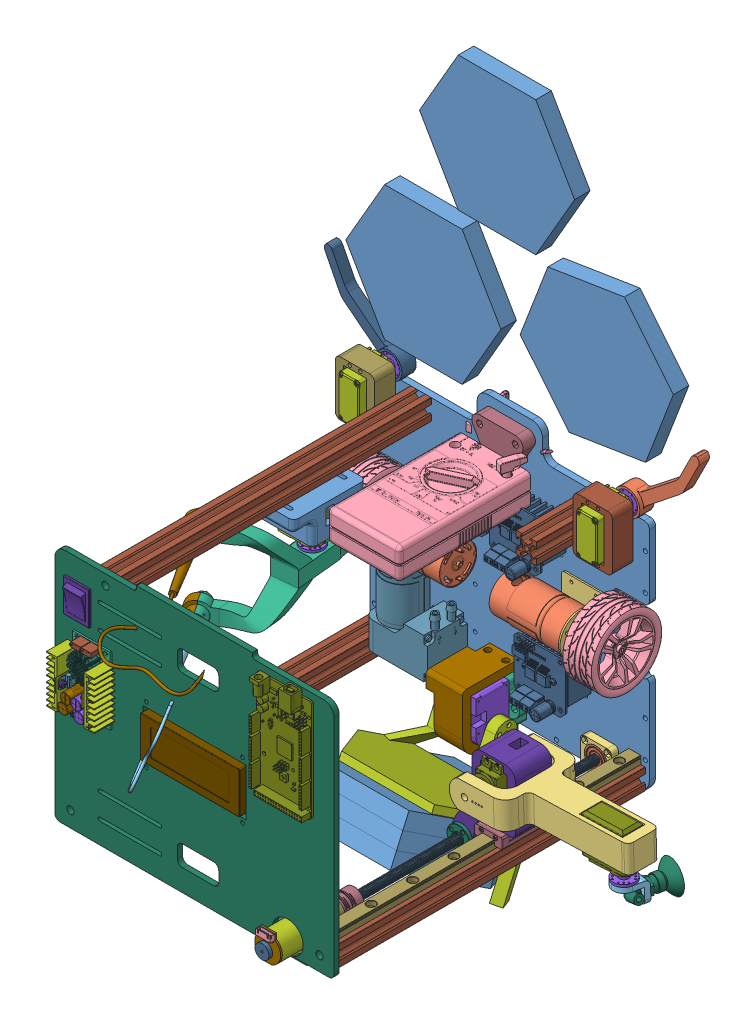
SolidWorks assembly conception_grand_robot_version_final, configuration Default. Lengths in mm.
Overall size (518.63 617.26 405.48).
409 component instances, 143 part files, 130 mates.
Components (placement in the parent):
- base-1: base [Default] at (122.9528 157.5833 221.7888) size (270 260 6)
- assemblage_motor_complet-1: assemblage_motor_complet [Default] at (122.8124 108.9997 302.4952) x (0 1 0) z (-1 0 0) size (92.56 92.56 113.78)
  - Motor 300RPM-1: Motor 300RPM [Default] at (60.9586 47.2064 18.9845) size (37 37 94.88)
  - BAse motor-1: BAse motor [Predeterminado] at (28.5836 74.7064 94.3595) x (1 0 0) z (0 0 -1) size (40 46 43)
  - wheel-1: wheel [Default] at (48.5836 55.7064 86.8847) x (-0.872522 -0.488575 0) z (-0.488575 0.872522 0) size (68 29.75 68)
  - accoupelement court-1: accoupelement court [Default] at (48.5836 55.7064 101.8595) x (-0.320714 0.947176 0) z (0 0 1) size (13.86 12 18)
- assemblage_motor_complet-2: assemblage_motor_complet [Default] at (123.0933 206.1669 302.4952) x (0 -1 0) z (1 0 0) size (92.56 92.56 113.78)
  - Motor 300RPM-1: Motor 300RPM [Default] at (60.9586 47.2064 18.9845) size (37 37 94.88)
  - BAse motor-1: BAse motor [Predeterminado] at (28.5836 74.7064 94.3595) x (1 0 0) z (0 0 -1) size (40 46 43)
  - wheel-1: wheel [Default] at (48.5836 55.7064 86.8847) x (-0.872522 -0.488575 0) z (-0.488575 0.872522 0) size (68 29.75 68)
  - accoupelement court-1: accoupelement court [Default] at (48.5836 55.7064 101.8595) x (-0.320714 0.947176 0) z (0 0 1) size (13.86 12 18)
- bille porteuse-1: bille porteuse [Défaut] at (122.9528 39.4366 218.2888) x (-1 0 0) z (0 1 0) size (52.5 22.5 43)
  - Robot2015_support bille porteuse_arriere-1: Robot2015_support bille porteuse_arriere [Défaut] at (0 9.5 0) size (52.5 22.5 43)
- pince 3-1: pince 3 [Default] at (122.9528 -18.4476 239.2747) x (1 0 0) z (0 0.403318 0.91506) size (152.18 120 85.13)
- Servo-1: Servo [Default] at (139.2028 54.0833 260.7888) x (0 0 -1) z (-1 0 0) size (32 43 41.5)
- TABLE_2021.step-1: TABLE_2021.step [Default] at (1982.9528 825.0833 212.7888) x (0 -1 0) z (0 0 1) size (3306.25 2336 1029.4) (hidden)
  - BaseTable.step-1: BaseTable.step [Défaut] at (0 0 -22) x (1 0 0) z (0 -1 0) size (3288 1022 2266)
    - Edge Beacon Right.step-1: Edge Beacon Right.step [Défaut] at (-884.0915 354.4211 0) x (1 0 0) z (0 1 0) size (122 122 92)
      - EdgeBeacons_Base.step-1: EdgeBeacons_Base.step [Défaut] at (3967.0915 -989 -332.4211) x (0 -1 0) z (1 0 0) size (122 22 122)
      - EdgeBeacons_SmallBorder.step-1: EdgeBeacons_SmallBorder.step [Défaut] at (4028.0915 -950 -332.4211) x (0 1 0) z (1 0 0) size (22 70 100)
      - EdgeBeacons_LargeBorder.step-1: EdgeBeacons_LargeBorder.step [Défaut] at (3906.0915 -1050 -332.4211) x (1 0 0) z (0 -1 0) size (22 70 122)
    - Edge Beacon Left.step-1: Edge Beacon Left.step [Défaut] at (-1609.4995 44.4467 0) x (1 0 0) z (0 1 0) size (122 122 92)
      - EdgeBeacons_Base.step-1: EdgeBeacons_Base.step [Défaut] at (1526.4995 -39 -44.4467) x (0 -1 0) z (-1 0 0) size (122 22 122)
      - EdgeBeacons_LargeBorder.step-1: EdgeBeacons_LargeBorder.step [Défaut] at (1565.4995 -100 -22.4467) x (1 0 0) z (0 -1 0) size (22 70 122)
      - EdgeBeacons_SmallBorder.step-1: EdgeBeacons_SmallBorder.step [Défaut] at (1465.4995 22 -22.4467) x (0 -1 0) z (-1 0 0) size (22 70 100)
    - Edge Beacon Right_1.step-1: Edge Beacon Right_1.step [Défaut] at (-884.0915 354.4211 0) x (1 0 0) z (0 1 0) size (122 122 92)
      - EdgeBeacons_Base.step-1: EdgeBeacons_Base.step [Défaut] at (3967.0915 -39 -332.4211) x (0 -1 0) z (1 0 0) size (122 22 122)
      - EdgeBeacons_SmallBorder.step-1: EdgeBeacons_SmallBorder.step [Défaut] at (4028.0915 0 -332.4211) x (0 1 0) z (1 0 0) size (22 70 100)
      - EdgeBeacons_LargeBorder.step-1: EdgeBeacons_LargeBorder.step [Défaut] at (3906.0915 -100 -332.4211) x (1 0 0) z (0 -1 0) size (22 70 122)
    - Edge Beacon Right_2.step-1: Edge Beacon Right_2.step [Défaut] at (-1546.4323 1056.5508 0) x (1 0 0) z (0 1 0) size (122 122 92)
      - EdgeBeacons_Base.step-1: EdgeBeacons_Base.step [Défaut] at (4629.4323 -1939 -1034.5508) x (0 -1 0) z (1 0 0) size (122 22 122)
      - EdgeBeacons_SmallBorder.step-1: EdgeBeacons_SmallBorder.step [Défaut] at (4690.4323 -1900 -1034.5508) x (0 1 0) z (1 0 0) size (22 70 100)
      - EdgeBeacons_LargeBorder.step-1: EdgeBeacons_LargeBorder.step [Défaut] at (4568.4323 -2000 -1034.5508) x (1 0 0) z (0 -1 0) size (22 70 122)
    - Edge Beacon Left_1.step-1: Edge Beacon Left_1.step [Défaut] at (-933.7648 1396.3534 0) x (1 0 0) z (0 1 0) size (122 122 92)
      - EdgeBeacons_Base.step-1: EdgeBeacons_Base.step [Défaut] at (850.7648 -1939 -1396.3534) x (0 -1 0) z (-1 0 0) size (122 22 122)
      - EdgeBeacons_LargeBorder.step-1: EdgeBeacons_LargeBorder.step [Défaut] at (889.7648 -2000 -1374.3534) x (1 0 0) z (0 -1 0) size (22 70 122)
      - EdgeBeacons_SmallBorder.step-1: EdgeBeacons_SmallBorder.step [Défaut] at (789.7648 -1878 -1374.3534) x (0 -1 0) z (-1 0 0) size (22 70 100)
    - Edge Beacon Left_2.step-1: Edge Beacon Left_2.step [Défaut] at (-2304.4911 1279.1137 0) x (1 0 0) z (0 1 0) size (122 122 92)
      - EdgeBeacons_Base.step-1: EdgeBeacons_Base.step [Défaut] at (2221.4911 -989 -1279.1137) x (0 -1 0) z (-1 0 0) size (122 22 122)
      - EdgeBeacons_LargeBorder.step-1: EdgeBeacons_LargeBorder.step [Défaut] at (2260.4911 -1050 -1257.1137) x (1 0 0) z (0 -1 0) size (22 70 122)
      - EdgeBeacons_SmallBorder.step-1: EdgeBeacons_SmallBorder.step [Défaut] at (2160.4911 -928 -1257.1137) x (0 -1 0) z (-1 0 0) size (22 70 100)
    - BorderLong.step-1: BorderLong.step [Défaut] at (0 0 -22) size (3000 92 22)
    - BorderLong.step-2: BorderLong.step [Défaut] at (3000 0 2022) x (-1 0 0) z (0 0 -1) size (3000 92 22)
    - BorderSmall.step-1: BorderSmall.step [Défaut] at (-22 0 2022) x (0 0 -1) z (1 0 0) size (2044 92 22)
    - BorderSmall.step-2: BorderSmall.step [Défaut] at (3022 0 -22) x (0 0 1) z (-1 0 0) size (2044 92 22)
    - Ground.step-1: Ground.step [Défaut] at origin size (3000 22 2000)
    - MiddleBeaconTop.step-1: MiddleBeaconTop.step [Défaut] at (1500 22 -122) size (400 22 200)
    - MiddleBeaconVertSupport1.step-1: MiddleBeaconVertSupport1.step [Défaut] at (1500 22 -22) x (0 0 1) z (-1 0 0) size (200 978 22)
    - MiddleBeaconVertSupport2.step-1: MiddleBeaconVertSupport2.step [Défaut] at (1600 22 -233) size (200 1000 22)
    - ExperimentZone.step-1: ExperimentZone.step [Défaut] at (225 92 -22) size (450 22 200)
    - ExperimentZone.step-2: ExperimentZone.step [Défaut] at (2775 92 -22) size (450 22 200)
    - PaintExperience.step-1: PaintExperience.step [Défaut] at (0 92 -22) size (450 0.1 22)
    - PaintExperience.step-2: PaintExperience.step [Défaut] at (2550 92 -22) size (450 0.1 22)
    - BaseTable-0.step-1: BaseTable-0.step [Défaut] at origin size (22 0.1 600)
    - BaseTable-1.step-1: BaseTable-1.step [Défaut] at origin size (22 0.1 600)
  - Echantillons.step-1: Echantillons.step [Défaut] at origin size (3292.15 1762.13 85)
    - EchantillonBleu.step-1: EchantillonBleu.step [Défaut] at (900 -555 0) x (0.5 0.866025 0) z (0 0 1) size (129.9 149.69 15)
    - EchantillonBleu.step-2: EchantillonBleu.step [Défaut] at (892.3031 -1292.3031 15) x (0.965926 0.258819 0) z (0 0 -1) size (129.9 149.69 15)
    - EchantillonBleu.step-3: EchantillonBleu.step [Défaut] at (2100 -555 0) x (0.5 0.866025 0) z (0 0 1) size (129.9 149.69 15)
    - EchantillonBleu.step-4: EchantillonBleu.step [Défaut] at (2113.9218 -1288.3769 15) x (0.34202 -0.939693 0) z (0 0 -1) size (129.9 149.69 15)
    - EchantillonVert.step-1: EchantillonVert.step [Défaut] at (2085.0581 -1446.2787 15) x (0.906308 0.422618 0) z (0 0 -1) size (129.9 149.69 15)
    - EchantillonRouge.step-1: EchantillonRouge.step [Défaut] at (1954.3221 -1366.4789 15) x (0.258819 0.965926 0) z (0 0 -1) size (129.9 149.69 15)
    - EchantillonVert.step-2: EchantillonVert.step [Défaut] at (830 -675 0) x (0.5 0.866025 0) z (0 0 1) size (129.9 149.69 15)
    - EchantillonRouge.step-2: EchantillonRouge.step [Défaut] at (900 -795 0) x (0.5 0.866025 0) z (0 0 1) size (129.9 149.69 15)
    - EchantillonVert.step-3: EchantillonVert.step [Défaut] at (2170 -675 0) x (0.5 0.866025 0) z (0 0 1) size (129.9 149.69 15)
    - EchantillonRouge.step-3: EchantillonRouge.step [Défaut] at (2100 -795 0) x (0.5 0.866025 0) z (0 0 1) size (129.9 149.69 15)
    - EchantillonVert.step-4: EchantillonVert.step [Défaut] at (1044.2641 -1329.1257 15) x (0.965926 -0.258819 0) z (0 0 -1) size (129.9 149.69 15)
    - EchantillonRouge.step-4: EchantillonRouge.step [Défaut] at (950 -1450 15) x (0.965926 0.258819 0) z (0 0 -1) size (129.9 149.69 15)
    - EchantillonBleu.step-5: EchantillonBleu.step [Défaut] at (311.5685 -1879.3503 70) x (0.258819 -0.965926 0) z (0 0 1) size (129.9 149.69 15)
    - EchantillonRouge.step-5: EchantillonRouge.step [Défaut] at (120.6497 -1688.4315 70) x (-0.258819 0.965926 0) z (0 0 1) size (129.9 149.69 15)
    - EchantillonBleu.step-6: EchantillonBleu.step [Défaut] at (2879.3503 -1688.4315 70) x (0.965926 0.258819 0) z (0 0 1) size (129.9 149.69 15)
    - EchantillonRouge.step-6: EchantillonRouge.step [Défaut] at (2688.4315 -1879.3503 70) x (-0.965926 -0.258819 0) z (0 0 1) size (129.9 149.69 15)
    - EchantillonVert.step-5: EchantillonVert.step [Défaut] at (-64.9519 -300 70) x (-0.5 0.866025 0) z (0 0 1) size (129.9 149.69 15)
    - EchantillonVert.step-6: EchantillonVert.step [Défaut] at (3064.9519 -300 70) size (129.9 149.69 15)
  - Frises.step-1: Frises.step [Défaut] at origin size (2100 194.46 292.81)
    - FriseJaune.step-1: FriseJaune.step [Défaut] at (810 0 0) x (0 -1 0) z (0 0 1) size (194.46 720 292.81)
      - Frise.step-1: Frise.step [Défaut] at origin size (194.46 720 292.81)
        - FRISE_2.step-1: FRISE_2.step [Défaut] at origin size (169.05 720 270.81)
        - BORDURE.step-1: BORDURE.step [Défaut] at origin size (41.05 720 49.11)
        - TRIANGLE_GAUCHE.step-1: TRIANGLE_GAUCHE.step [Défaut] at origin size (40.41 22 70)
        - TRIANGLE_DROIT.step-1: TRIANGLE_DROIT.step [Défaut] at origin size (40.41 22 70)
        - TRIANGLE_CENTRE.step-1: TRIANGLE_CENTRE.step [Défaut] at origin size (40.41 22 70)
        - TaquetArriere.step-1: TaquetArriere.step [Défaut] at origin size (22 22 168.21)
        - TaquetArriere.step-2: TaquetArriere.step [Défaut] at (0 698 0) size (22 22 168.21)
        - TaquetArriere.step-3: TaquetArriere.step [Défaut] at (0 349 0) size (22 22 168.21)
      - FriseJaune-2.step-1: FriseJaune-2.step [Défaut] at origin size (150.01 720 259.81)
    - FriseViolet.step-1: FriseViolet.step [Défaut] at (2190 0 0) x (0 -1 0) z (0 0 1) size (194.46 720 292.81)
      - Frise_1.step-1: Frise_1.step [Défaut] at origin size (194.46 720 292.81)
        - FRISE_2.step-1: FRISE_2.step [Défaut] at origin size (169.05 720 270.81)
        - BORDURE.step-1: BORDURE.step [Défaut] at origin size (41.05 720 49.11)
        - TRIANGLE_GAUCHE.step-1: TRIANGLE_GAUCHE.step [Défaut] at origin size (40.41 22 70)
        - TRIANGLE_DROIT.step-1: TRIANGLE_DROIT.step [Défaut] at origin size (40.41 22 70)
        - TRIANGLE_CENTRE.step-1: TRIANGLE_CENTRE.step [Défaut] at origin size (40.41 22 70)
        - TaquetArriere.step-1: TaquetArriere.step [Défaut] at origin size (22 22 168.21)
        - TaquetArriere.step-2: TaquetArriere.step [Défaut] at (0 698 0) size (22 22 168.21)
        - TaquetArriere.step-3: TaquetArriere.step [Défaut] at (0 349 0) size (22 22 168.21)
      - FriseViolet-3.step-1: FriseViolet-3.step [Défaut] at origin size (150.01 720 259.81)
  - Distributeurs.step-1: Distributeurs.step [Défaut] at origin size (3259.81 2051.07 183.14)
    - Distributeur 2 Side.step-1: Distributeur 2 Side.step [Défaut] at (11 -1250 0) x (0 1 0) z (1 0 0) size (187.35 183.14 137.52)
      - TasseauBordure.step-1: TasseauBordure.step [Défaut] at origin size (106 22 22)
      - TasseauCote.step-1: TasseauCote.step [Défaut] at (-64 0 29) size (22 22 80)
      - TasseauCote.step-2: TasseauCote.step [Défaut] at (64 0 29) size (22 22 80)
      - TasseauAvant.step-1: TasseauAvant.step [Défaut] at (0 0 80) size (150 22 22)
      - EchantillonBleu.step-1: EchantillonBleu.step [Défaut] at (0 59.0455 -5.9792) x (0.866025 0.454532 -0.208327) z (0 0.416655 0.909065) size (129.9 149.69 15)
      - EchantillonVert.step-1: EchantillonVert.step [Défaut] at (0 59.0455 10.5213) x (0.866025 0.454532 -0.208327) z (0 0.416655 0.909065) size (129.9 149.69 15)
      - EchantillonRouge.step-1: EchantillonRouge.step [Défaut] at (0 59.0455 27.0218) x (0.866025 0.454532 -0.208327) z (0 0.416655 0.909065) size (129.9 149.69 15)
    - Distributeur 2 Side_1.step-1: Distributeur 2 Side_1.step [Défaut] at (2989 -1250 0) x (0 -1 0) z (-1 0 0) size (187.35 183.14 137.52)
      - TasseauBordure.step-1: TasseauBordure.step [Défaut] at origin size (106 22 22)
      - TasseauCote.step-1: TasseauCote.step [Défaut] at (-64 0 29) size (22 22 80)
      - TasseauCote.step-2: TasseauCote.step [Défaut] at (64 0 29) size (22 22 80)
      - TasseauAvant.step-1: TasseauAvant.step [Défaut] at (0 0 80) size (150 22 22)
      - EchantillonBleu.step-1: EchantillonBleu.step [Défaut] at (0 59.0455 -5.9792) x (0.866025 0.454532 -0.208327) z (0 0.416655 0.909065) size (129.9 149.69 15)
      - EchantillonVert.step-1: EchantillonVert.step [Défaut] at (0 59.0455 10.5213) x (0.866025 0.454532 -0.208327) z (0 0.416655 0.909065) size (129.9 149.69 15)
      - EchantillonRouge.step-1: EchantillonRouge.step [Défaut] at (0 59.0455 27.0218) x (0.866025 0.454532 -0.208327) z (0 0.416655 0.909065) size (129.9 149.69 15)
    - Distributeur 2 Top.step-1: Distributeur 2 Top.step [Défaut] at (1650 -11 0) x (1 0 0) z (0 -1 0) size (187.35 183.14 137.52)
      - TasseauBordure_1.step-1: TasseauBordure_1.step [Défaut] at origin size (106 22 22)
      - TasseauCote_1.step-1: TasseauCote_1.step [Défaut] at (-64 0 29) size (22 22 80)
      - TasseauCote_1.step-2: TasseauCote_1.step [Défaut] at (64 0 29) size (22 22 80)
      - TasseauAvant_1.step-1: TasseauAvant_1.step [Défaut] at (0 0 80) size (150 22 22)
      - EchantillonBleu.step-1: EchantillonBleu.step [Défaut] at (0 59.0455 27.0218) x (0.866025 0.454532 -0.208327) z (0 0.416655 0.909065) size (129.9 149.69 15)
      - EchantillonRouge.step-1: EchantillonRouge.step [Défaut] at (0 59.0455 -5.9792) x (0.866025 0.454532 -0.208327) z (0 0.416655 0.909065) size (129.9 149.69 15)
      - EchantillonVert.step-1: EchantillonVert.step [Défaut] at (0 59.0455 10.5213) x (0.866025 0.454532 -0.208327) z (0 0.416655 0.909065) size (129.9 149.69 15)
    - Distributeur 2 Top_1.step-1: Distributeur 2 Top_1.step [Défaut] at (1350 -11 0) x (1 0 0) z (0 -1 0) size (187.35 183.14 137.52)
      - TasseauBordure_1.step-1: TasseauBordure_1.step [Défaut] at origin size (106 22 22)
      - TasseauCote_1.step-1: TasseauCote_1.step [Défaut] at (-64 0 29) size (22 22 80)
      - TasseauCote_1.step-2: TasseauCote_1.step [Défaut] at (64 0 29) size (22 22 80)
      - TasseauAvant_1.step-1: TasseauAvant_1.step [Défaut] at (0 0 80) size (150 22 22)
      - EchantillonBleu.step-1: EchantillonBleu.step [Défaut] at (0 59.0455 27.0218) x (0.866025 0.454532 -0.208327) z (0 0.416655 0.909065) size (129.9 149.69 15)
      - EchantillonRouge.step-1: EchantillonRouge.step [Défaut] at (0 59.0455 -5.9792) x (0.866025 0.454532 -0.208327) z (0 0.416655 0.909065) size (129.9 149.69 15)
      - EchantillonVert.step-1: EchantillonVert.step [Défaut] at (0 59.0455 10.5213) x (0.866025 0.454532 -0.208327) z (0 0.416655 0.909065) size (129.9 149.69 15)
    - DistributeurCoin.step-1: DistributeurCoin.step [Défaut] at (0 -2000 175) size (525.56 525.56 44)
      - Taquet.step-1: Taquet.step [Défaut] at (0 0 -197) size (510 510 22)
      - SupportStatuette.step-1: SupportStatuette.step [Défaut] at (0 0 -197) size (169.71 169.71 22)
      - Taquet (1).step-1: Taquet (1).step [Défaut] at (0 0 -197) size (355.85 355.85 22)
    - DistributeurCoin_1.step-1: DistributeurCoin_1.step [Défaut] at (3000 -2000 300) x (0 1 0) z (0 0 1) size (525.56 525.56 44)
      - Taquet.step-1: Taquet.step [Défaut] at (0 0 -322) size (510 510 22)
      - SupportStatuette.step-1: SupportStatuette.step [Défaut] at (0 0 -322) size (169.71 169.71 22)
      - Taquet (1).step-1: Taquet (1).step [Défaut] at (0 0 -322) size (355.85 355.85 22)
    - DistributeurBordure.step-1: DistributeurBordure.step [Défaut] at (-200 -250 0) size (107.9 150 92)
      - Support (1).step-1: Support (1).step [Défaut] at (200 -50 -22) size (107.9 150 22)
      - Equerre.step-1: Equerre.step [Défaut] at (200 -50 -22) size (70 22 70)
    - DistributeurBordure_1.step-1: DistributeurBordure_1.step [Défaut] at (3250 -250 0) x (-1 0 0) z (0 0 1) size (107.9 150 92)
      - Support (1).step-1: Support (1).step [Défaut] at (250 50 -22) size (107.9 150 22)
      - Equerre.step-1: Equerre.step [Défaut] at (250 50 -22) size (70 22 70)
  - CarreFouille.step-1: CarreFouille.step [Défaut] at origin size (1850 85.95 153.3)
    - CarreFouilleTresorJaune.step-1: CarreFouilleTresorJaune.step [Défaut] at (667.5 -2000 0) x (0 -1 0) z (0 0 1) size (85.95 185 153.3)
      - CarreFouille_1.step-1: CarreFouille_1.step [Défaut] at (64.8942 -232.3942 0) size (85.94 185 153.3)
        - PCB_datation.step-1: PCB_datation.step [Défaut] at (0 0 158.7231) x (0 1 0) z (0 0 1) size (100 19.02 9.26)
          - PCB Component.step-1: PCB Component.step [Défaut] at (232.3942 48.7058 -10.7729) x (1 0 0) z (0 0.390731 0.920505) size (100 20 1.57)
            - Board.step-1: Board.step [Défaut] at origin size (100 20 1.57)
        - BASE.step-1: BASE.step [Défaut] at (-27.8942 232.3942 35) size (15 185 70)
        - LEFT_ARM.step-1: LEFT_ARM.step [Défaut] at (-27.8942 232.3942 35) size (55 15 70)
        - RIGHT_ARM.step-1: RIGHT_ARM.step [Défaut] at (-27.8942 232.3942 35) size (55 15 70)
        - SQUARE.step-1: SQUARE.step [Défaut] at (-31.092 232.3942 20.7181) x (0.920505 0 0.390731) z (-0.390731 0 0.920505) size (22 150 150)
      - CarreFouilleTresorJaune-4.step-1: CarreFouilleTresorJaune-4.step [Défaut] at origin size (58.62 150 138.08)
      - CarreFouilleTresorJaune-5.step-1: CarreFouilleTresorJaune-5.step [Défaut] at origin size (58.62 150 138.08)
    - CarreFouilleRadioactif.step-1: CarreFouilleRadioactif.step [Défaut] at (1037.5 -2000 0) x (0 -1 0) z (0 0 1) size (85.95 185 153.3)
      - CarreFouille_2.step-1: CarreFouille_2.step [Défaut] at (364.8942 -102.3942 0) size (85.94 185 153.3)
        - PCB_datation_1.step-1: PCB_datation_1.step [Défaut] at (0 0 158.7231) x (0 1 0) z (0 0 1) size (100 19.02 9.26)
          - PCB Component_1.step-1: PCB Component_1.step [Défaut] at (102.3942 348.7058 -10.7729) x (1 0 0) z (0 0.390731 0.920505) size (100 20 1.57)
            - Board.step-1: Board.step [Défaut] at origin size (100 20 1.57)
        - BASE.step-1: BASE.step [Défaut] at (-327.8942 102.3942 35) size (15 185 70)
        - LEFT_ARM.step-1: LEFT_ARM.step [Défaut] at (-327.8942 102.3942 35) size (55 15 70)
        - RIGHT_ARM.step-1: RIGHT_ARM.step [Défaut] at (-327.8942 102.3942 35) size (55 15 70)
        - SQUARE.step-1: SQUARE.step [Défaut] at (-331.092 102.3942 20.7181) x (0.920505 0 0.390731) z (-0.390731 0 0.920505) size (22 150 150)
      - CarreFouilleRadioactif-6.step-1: CarreFouilleRadioactif-6.step [Défaut] at origin size (58.62 150 138.08)
      - CarreFouilleRadioactif-7.step-1: CarreFouilleRadioactif-7.step [Défaut] at origin size (58.62 150 138.08)
    - CarreFouilleTresorJaune_1.step-1: CarreFouilleTresorJaune_1.step [Défaut] at (852.5 -2000 0) x (0 -1 0) z (0 0 1) size (85.95 185 153.3)
      - CarreFouille_3.step-1: CarreFouille_3.step [Défaut] at (264.8942 282.6058 0) size (85.94 185 153.3)
        - PCB_datation_2.step-1: PCB_datation_2.step [Défaut] at (0 0 158.7231) x (0 1 0) z (0 0 1) size (100 19.02 9.26)
          - PCB Component_2.step-1: PCB Component_2.step [Défaut] at (-282.6058 248.7058 -10.7729) x (1 0 0) z (0 0.390731 0.920505) size (100 20 1.57)
            - Board.step-1: Board.step [Défaut] at origin size (100 20 1.57)
        - BASE.step-1: BASE.step [Défaut] at (-227.8942 -282.6058 35) size (15 185 70)
        - LEFT_ARM.step-1: LEFT_ARM.step [Défaut] at (-227.8942 -282.6058 35) size (55 15 70)
        - RIGHT_ARM.step-1: RIGHT_ARM.step [Défaut] at (-227.8942 -282.6058 35) size (55 15 70)
        - SQUARE.step-1: SQUARE.step [Défaut] at (-231.092 -282.6058 20.7181) x (0.920505 0 0.390731) z (-0.390731 0 0.920505) size (22 150 150)
      - CarreFouilleTresorJaune_1-8.step-1: CarreFouilleTresorJaune_1-8.step [Défaut] at origin size (58.62 150 138.08)
      - CarreFouilleTresorJaune_1-9.step-1: CarreFouilleTresorJaune_1-9.step [Défaut] at origin size (58.62 150 138.08)
    - CarreFouilleTresorViolet.step-1: CarreFouilleTresorViolet.step [Défaut] at (1222.5 -2000 0) x (0 -1 0) z (0 0 1) size (85.95 185 153.3)
      - CarreFouille_4.step-1: CarreFouille_4.step [Défaut] at (464.8942 112.6058 0) size (85.94 185 153.3)
        - PCB_datation_3.step-1: PCB_datation_3.step [Défaut] at (0 0 158.7231) x (0 1 0) z (0 0 1) size (100 19.02 9.26)
          - PCB Component_3.step-1: PCB Component_3.step [Défaut] at (-112.6058 448.7058 -10.7729) x (1 0 0) z (0 0.390731 0.920505) size (100 20 1.57)
            - Board.step-1: Board.step [Défaut] at origin size (100 20 1.57)
        - BASE.step-1: BASE.step [Défaut] at (-427.8942 -112.6058 35) size (15 185 70)
        - LEFT_ARM.step-1: LEFT_ARM.step [Défaut] at (-427.8942 -112.6058 35) size (55 15 70)
        - RIGHT_ARM.step-1: RIGHT_ARM.step [Défaut] at (-427.8942 -112.6058 35) size (55 15 70)
        - SQUARE.step-1: SQUARE.step [Défaut] at (-431.092 -112.6058 20.7181) x (0.920505 0 0.390731) z (-0.390731 0 0.920505) size (22 150 150)
      - CarreFouilleTresorViolet-10.step-1: CarreFouilleTresorViolet-10.step [Défaut] at origin size (58.62 150 138.08)
      - CarreFouilleTresorViolet-11.step-1: CarreFouilleTresorViolet-11.step [Défaut] at origin size (58.62 150 138.08)
    - CarreFouilleTresorJaune_2.step-1: CarreFouilleTresorJaune_2.step [Défaut] at (1407.5 -2000 0) x (0 -1 0) z (0 0 1) size (85.95 185 153.3)
      - CarreFouille_5.step-1: CarreFouille_5.step [Défaut] at (464.8942 27.6058 0) size (85.94 185 153.3)
        - PCB_datation_4.step-1: PCB_datation_4.step [Défaut] at (0 0 158.7231) x (0 1 0) z (0 0 1) size (100 19.02 9.26)
          - PCB Component_4.step-1: PCB Component_4.step [Défaut] at (-27.6058 448.7058 -10.7729) x (1 0 0) z (0 0.390731 0.920505) size (100 20 1.57)
            - Board.step-1: Board.step [Défaut] at origin size (100 20 1.57)
        - BASE.step-1: BASE.step [Défaut] at (-427.8942 -27.6058 35) size (15 185 70)
        - LEFT_ARM.step-1: LEFT_ARM.step [Défaut] at (-427.8942 -27.6058 35) size (55 15 70)
        - RIGHT_ARM.step-1: RIGHT_ARM.step [Défaut] at (-427.8942 -27.6058 35) size (55 15 70)
        - SQUARE.step-1: SQUARE.step [Défaut] at (-431.092 -27.6058 20.7181) x (0.920505 0 0.390731) z (-0.390731 0 0.920505) size (22 150 150)
      - CarreFouilleTresorJaune_2-12.step-1: CarreFouilleTresorJaune_2-12.step [Défaut] at origin size (58.62 150 138.08)
      - CarreFouilleTresorJaune_2-13.step-1: CarreFouilleTresorJaune_2-13.step [Défaut] at origin size (58.62 150 138.08)
    - CarreFouilleTresorViolet_1.step-1: CarreFouilleTresorViolet_1.step [Défaut] at (1777.5 -2000 0) x (0 -1 0) z (0 0 1) size (85.95 185 153.3)
      - CarreFouille_6.step-1: CarreFouille_6.step [Défaut] at (664.8942 -42.3942 0) size (85.94 185 153.3)
        - PCB_datation_5.step-1: PCB_datation_5.step [Défaut] at (0 0 158.7231) x (0 1 0) z (0 0 1) size (100 19.02 9.26)
          - PCB Component_5.step-1: PCB Component_5.step [Défaut] at (42.3942 648.7058 -10.7729) x (1 0 0) z (0 0.390731 0.920505) size (100 20 1.57)
            - Board.step-1: Board.step [Défaut] at origin size (100 20 1.57)
        - BASE.step-1: BASE.step [Défaut] at (-627.8942 42.3942 35) size (15 185 70)
        - LEFT_ARM.step-1: LEFT_ARM.step [Défaut] at (-627.8942 42.3942 35) size (55 15 70)
        - RIGHT_ARM.step-1: RIGHT_ARM.step [Défaut] at (-627.8942 42.3942 35) size (55 15 70)
        - SQUARE.step-1: SQUARE.step [Défaut] at (-631.092 42.3942 20.7181) x (0.920505 0 0.390731) z (-0.390731 0 0.920505) size (22 150 150)
      - CarreFouilleTresorViolet_1-14.step-1: CarreFouilleTresorViolet_1-14.step [Défaut] at origin size (58.62 150 138.08)
      - CarreFouilleTresorViolet_1-15.step-1: CarreFouilleTresorViolet_1-15.step [Défaut] at origin size (58.62 150 138.08)
    - CarreFouilleTresorJaune_3.step-1: CarreFouilleTresorJaune_3.step [Défaut] at (1592.5 -2000 0) x (0 -1 0) z (0 0 1) size (85.95 185 153.3)
      - CarreFouille_7.step-1: CarreFouille_7.step [Défaut] at (464.8942 242.6058 0) size (85.94 185 153.3)
        - PCB_datation_6.step-1: PCB_datation_6.step [Défaut] at (0 0 158.7231) x (0 1 0) z (0 0 1) size (100 19.02 9.26)
          - PCB Component_6.step-1: PCB Component_6.step [Défaut] at (-242.6058 448.7058 -10.7729) x (1 0 0) z (0 0.390731 0.920505) size (100 20 1.57)
            - Board.step-1: Board.step [Défaut] at origin size (100 20 1.57)
        - BASE.step-1: BASE.step [Défaut] at (-427.8942 -242.6058 35) size (15 185 70)
        - LEFT_ARM.step-1: LEFT_ARM.step [Défaut] at (-427.8942 -242.6058 35) size (55 15 70)
        - RIGHT_ARM.step-1: RIGHT_ARM.step [Défaut] at (-427.8942 -242.6058 35) size (55 15 70)
        - SQUARE.step-1: SQUARE.step [Défaut] at (-431.092 -242.6058 20.7181) x (0.920505 0 0.390731) z (-0.390731 0 0.920505) size (22 150 150)
      - CarreFouilleTresorJaune_3-16.step-1: CarreFouilleTresorJaune_3-16.step [Défaut] at origin size (58.62 150 138.08)
      - CarreFouilleTresorJaune_3-17.step-1: CarreFouilleTresorJaune_3-17.step [Défaut] at origin size (58.62 150 138.08)
    - CarreFouilleTresorViolet_2.step-1: CarreFouilleTresorViolet_2.step [Défaut] at (2147.5 -2000 0) x (0 -1 0) z (0 0 1) size (85.95 185 153.3)
      - CarreFouille_8.step-1: CarreFouille_8.step [Défaut] at (564.8942 -12.3942 0) size (85.94 185 153.3)
        - PCB_datation_7.step-1: PCB_datation_7.step [Défaut] at (0 0 158.7231) x (0 1 0) z (0 0 1) size (100 19.02 9.26)
          - PCB Component_7.step-1: PCB Component_7.step [Défaut] at (12.3942 548.7058 -10.7729) x (1 0 0) z (0 0.390731 0.920505) size (100 20 1.57)
            - Board.step-1: Board.step [Défaut] at origin size (100 20 1.57)
        - BASE.step-1: BASE.step [Défaut] at (-527.8942 12.3942 35) size (15 185 70)
        - LEFT_ARM.step-1: LEFT_ARM.step [Défaut] at (-527.8942 12.3942 35) size (55 15 70)
        - RIGHT_ARM.step-1: RIGHT_ARM.step [Défaut] at (-527.8942 12.3942 35) size (55 15 70)
        - SQUARE.step-1: SQUARE.step [Défaut] at (-531.092 12.3942 20.7181) x (0.920505 0 0.390731) z (-0.390731 0 0.920505) size (22 150 150)
      - CarreFouilleTresorViolet_2-18.step-1: CarreFouilleTresorViolet_2-18.step [Défaut] at origin size (58.62 150 138.08)
      - CarreFouilleTresorViolet_2-19.step-1: CarreFouilleTresorViolet_2-19.step [Défaut] at origin size (58.62 150 138.08)
    - CarreFouilleRadioactif_1.step-1: CarreFouilleRadioactif_1.step [Défaut] at (1962.5 -2000 0) x (0 -1 0) z (0 0 1) size (85.95 185 153.3)
      - CarreFouille_9.step-1: CarreFouille_9.step [Défaut] at (564.8942 172.6058 0) size (85.94 185 153.3)
        - PCB_datation_8.step-1: PCB_datation_8.step [Défaut] at (0 0 158.7231) x (0 1 0) z (0 0 1) size (100 19.02 9.26)
          - PCB Component_8.step-1: PCB Component_8.step [Défaut] at (-172.6058 548.7058 -10.7729) x (1 0 0) z (0 0.390731 0.920505) size (100 20 1.57)
            - Board.step-1: Board.step [Défaut] at origin size (100 20 1.57)
        - BASE.step-1: BASE.step [Défaut] at (-527.8942 -172.6058 35) size (15 185 70)
        - LEFT_ARM.step-1: LEFT_ARM.step [Défaut] at (-527.8942 -172.6058 35) size (55 15 70)
        - RIGHT_ARM.step-1: RIGHT_ARM.step [Défaut] at (-527.8942 -172.6058 35) size (55 15 70)
        - SQUARE.step-1: SQUARE.step [Défaut] at (-531.092 -172.6058 20.7181) x (0.920505 0 0.390731) z (-0.390731 0 0.920505) size (22 150 150)
      - CarreFouilleRadioactif_1-20.step-1: CarreFouilleRadioactif_1-20.step [Défaut] at origin size (58.62 150 138.08)
      - CarreFouilleRadioactif_1-21.step-1: CarreFouilleRadioactif_1-21.step [Défaut] at origin size (58.62 150 138.08)
    - CarreFouilleTresorViolet_3.step-1: CarreFouilleTresorViolet_3.step [Défaut] at (2332.5 -2000 0) x (0 -1 0) z (0 0 1) size (85.95 185 153.3)
      - CarreFouille_10.step-1: CarreFouille_10.step [Défaut] at (564.8942 102.6058 0) size (85.94 185 153.3)
        - PCB_datation_9.step-1: PCB_datation_9.step [Défaut] at (0 0 158.7231) x (0 1 0) z (0 0 1) size (100 19.02 9.26)
          - PCB Component_9.step-1: PCB Component_9.step [Défaut] at (-102.6058 548.7058 -10.7729) x (1 0 0) z (0 0.390731 0.920505) size (100 20 1.57)
            - Board.step-1: Board.step [Défaut] at origin size (100 20 1.57)
        - BASE.step-1: BASE.step [Défaut] at (-527.8942 -102.6058 35) size (15 185 70)
        - LEFT_ARM.step-1: LEFT_ARM.step [Défaut] at (-527.8942 -102.6058 35) size (55 15 70)
        - RIGHT_ARM.step-1: RIGHT_ARM.step [Défaut] at (-527.8942 -102.6058 35) size (55 15 70)
        - SQUARE.step-1: SQUARE.step [Défaut] at (-531.092 -102.6058 20.7181) x (0.920505 0 0.390731) z (-0.390731 0 0.920505) size (22 150 150)
      - CarreFouilleTresorViolet_3-22.step-1: CarreFouilleTresorViolet_3-22.step [Défaut] at origin size (58.62 150 138.08)
      - CarreFouilleTresorViolet_3-23.step-1: CarreFouilleTresorViolet_3-23.step [Défaut] at origin size (58.62 150 138.08)
  - BarreSeparation.step-1: BarreSeparation.step [Défaut] at (1500 0 0) x (0 -1 0) z (0 0 1) size (300 22 22)
- support_servo-1: support_servo [Default] at (106.7028 59.8468 231.7888) x (0 1 0) z (1 0 0) size (59 53.86 35.5)
- BillePorteuse-1: BillePorteuse [Défaut] at (122.9528 54.0833 220.2888) x (-0.69086 0.722989 0) z (-0.722989 -0.69086 0) size (31 21.5 31)
- system element de jeu vertical_vf-1: system element de jeu vertical_vf [Default] at (217.6572 -298.0292 -19.4905) x (-1 0 0) z (0 1 0) size (196.65 333.36 101) (flexible)
  - FORSETI_PERFIL_20x20_V-SLOT-1: FORSETI_PERFIL_20x20_V-SLOT [Valor predeterminado] at (-26.2956 397.2794 339.6125) x (0 0 1) z (0 -1 0) size (20 20 300)
  - MGN_12_H_RAIL-1: MGN_12_H_RAIL [Default] at (-20.2956 247.2794 349.6125) x (-1 0 0) z (0 1 0) size (12 8 300)
  - MGN12H, LINEAR GUIDE BLOCK-1: MGN12H, LINEAR GUIDE BLOCK [Default] at (-26.2956 366.3254 355.1125) x (-1 0 0) z (0 1 0) size (27 10 47.52)
  - tige 8 mm-1: tige 8 mm [Varsayılan] at (4.532 245.0002 339.6125) x (0.955698 0 -0.294348) z (0.294348 0 0.955698) size (8.04 264.47 9.24)
  - ecrou 8mm-1: ecrou 8mm [Default] at (4.532 387.3254 339.6125) x (-0.858833 0 -0.512256) z (0 1 0) size (22 22 16.4)
  - 12V 350RPM Small DFRobot Motor v8.step-1: 12V 350RPM Small DFRobot Motor v8.step [Default] at (4.532 570.0002 339.6125) x (-1 0 0) z (0 -1 0) size (25 28.09 71.15)
    - B6B-XH-AM v6.step-1: B6B-XH-AM v6.step [Default] at (0 -26 0) size (14.01 6.15 4.63)
      - Component16.step-1: Component16.step [Default] at origin size (14.01 6.15 4.63)
        - Component9.step-1: Component9.step [Default] at (5.275 15.8465 -4.0011) x (-1 0 0) z (0 0 -1) size (0.52 0.52 2.82)
        - Component12.step-1: Component12.step [Default] at (5.275 15.8465 -4.0011) x (-1 0 0) z (0 0 -1) size (0.52 0.52 2.82)
        - Component13.step-1: Component13.step [Default] at (5.275 15.8465 -4.0011) x (-1 0 0) z (0 0 -1) size (0.52 0.52 2.82)
        - Component14.step-1: Component14.step [Default] at (5.275 15.8465 -4.0011) x (-1 0 0) z (0 0 -1) size (0.52 0.52 2.82)
        - Component10.step-1: Component10.step [Default] at (5.275 15.8465 -4.0011) x (-1 0 0) z (0 0 -1) size (0.52 0.52 2.82)
        - Component11.step-1: Component11.step [Default] at (5.275 15.8465 -4.0011) x (-1 0 0) z (0 0 -1) size (0.52 0.52 2.82)
        - Main.step-1: Main.step [Default] at (5.275 16.6906 -3.9287) x (-1 0 0) z (0 -1 0) size (14.01 4.63 5.64)
    - Shaft.step-1: Shaft.step [Default] at origin size (4 4 12)
    - Shaft_Coller.step-1: Shaft_Coller.step [Default] at origin size (7 7 2.5)
    - Body_Back.step-1: Body_Back.step [Default] at origin size (25 25 31)
    - Body_Front.step-1: Body_Front.step [Default] at origin size (25 25 21)
    - PCB.step-1: PCB.step [Default] at origin size (25 27.59 7.15)
    - EncoderMagnet.step-1: EncoderMagnet.step [Default] at origin size (13.5 13.5 3.5)
    - Text.step-1: Text.step [Default] at origin size (11.44 3.52 0.02)
  - support moteur 1-1: support moteur 1 [Default] at (4.532 547.2794 339.6125) x (1 0 0) z (0 -1 0) size (20.83 40 30)
  - NEMA17_Coupler-1: NEMA17_Coupler [Default] at (4.532 514.0002 339.6125) x (-0.068054 0 -0.997682) z (-0.997682 0 0.068054) size (26.77 26 23.11)
  - support moteur 2-2: support moteur 2 [Default] at (4.532 517.2794 339.6125) x (-1 0 0) z (0 1 0) size (20 40 30)
  - ventouse_final-1: ventouse_final [Default] at (-151.8807 336.7097 360.8717) x (0.287779 -0.052748 0.956243) z (-0.936783 0.192022 0.292515) size (30 42.25 32)
  - kiso-1: kiso [Predeterminado] at (-26.2956 373.6354 391.6125) x (0 0 -1) z (1 0 0) size (53.82 44.84 19.95)
  - support servo principale-2: support servo principale [Default] at (-26.2956 353.8254 391.6125) x (0 0 1) z (0 1 0) size (92 62.83 35)
  - Roulement_d3xd10xe4-1: Roulement_d3xd10xe4 [Défaut] at (-26.2956 351.1254 401.8625) x (0 -1 0) z (-0.546944 0 0.837169) size (5 13 13)
- hexagone-1: hexagone [Default] at (122.9528 9.7808 303.3201) x (1 0 0) z (0 -0.91506 0.403318) size (150 129.9 15)
- hexagone-2: hexagone [Default] at (122.9528 -17.671 315.4196) x (-1 0 0) z (0 0.91506 -0.403318) size (150 129.9 15)
- hexagone-3: hexagone [Default] at (122.9528 -17.671 315.4196) x (1 0 0) z (0 -0.91506 0.403318) size (150 129.9 15)
- roulement-1: roulement [Défaut] at (213.1252 41.5833 231.2888) x (0 0 1) z (-1 0 0) size (7 22 22)
- support_roullement-1: support_roullement [Default] at (213.1252 41.5833 234.7888) x (0 -1 0) z (0 0 -1) size (28 30 7)
- multimeter-1: multimeter [Default] at (122.9528 226.7833 296.6231) x (0 0 1) z (-1 0 0) size (180.84 43.58 76.59)
- sonde --1: sonde - [Default] at (51.5259 217.2637 431.4264) x (-0.524646 -0.145902 -0.838725) z (0.086283 0.971018 -0.222888) size (215.76 23.74 73.86)
- support_sonde-1: support_sonde [Default] at (-0.2607 149.7833 401.8495) x (0 -1 0) z (-0.846069 0 0.533074) size (93.66 119.92 95.94)
- Servo noir-1: Servo noir [По умолчанию] at (36.9528 232.5833 342.7888) x (-1 0 0) z (0 0 1) size (53 41.52 20)
- piece de liaison cercle MG996r-1: piece de liaison cercle MG996r [Défaut] at (46.9528 194.5833 342.7888) x (0.858553 0 0.512724) z (0 -1 0) size (20.75 20.75 5.3)
- sonde +-2: sonde + [Default] at (84.7897 203.1447 390.689) x (-0.596536 0.008342 -0.802543) z (-0.780413 0.227396 0.582449) size (216.04 15 75.5)
- FORSETI_PERFIL_20x20_V-SLOT-4: FORSETI_PERFIL_20x20_V-SLOT [Valor predeterminado] at (208.9528 247.5833 377.7888) x (0 1 0) z (0 0 1) size (20 20 300)
- Servo noir-3: Servo noir [По умолчанию] at (237.9528 256.0833 269.0888) x (0 -1 0) z (1 0 0) size (53 41.52 20)
- piece de liaison cercle MG996r-3: piece de liaison cercle MG996r [Défaut] at (237.9528 266.0833 228.0888) x (0.443122 0.896461 0) z (0 0 -1) size (20.75 20.75 5.3)
- FORSETI_PERFIL_20x20_V-SLOT-5: FORSETI_PERFIL_20x20_V-SLOT [Valor predeterminado] at (2.9528 42.5833 377.7888) x (0 1 0) z (0 0 1) size (20 20 300)
- IBT-2 (module only)-1: IBT-2 (module only) [Default] at (152.4528 207.7333 250.7888) x (-1 0 0) z (0 1 0) size (51 40.62 49.7)
- IBT-2 (module only)-2: IBT-2 (module only) [Default] at (93.4528 207.7333 245.3893) x (1 0 0) z (0 1 0) size (51 40.62 49.7)
- FORSETI_PERFIL_20x20_V-SLOT-6: FORSETI_PERFIL_20x20_V-SLOT [Valor predeterminado] at (36.9528 247.5833 377.7888) x (0 1 0) z (0 0 -1) size (20 20 300)
- support_servo_pince_lamen_imin-1: support_servo_pince_lamen_imin [Default] at (237.9528 256.0833 242.5888) size (38 53 20)
- Servo noir-4: Servo noir [По умолчанию] at (7.9528 256.0833 269.0888) x (0 -1 0) z (1 0 0) size (53 41.52 20)
- piece de liaison cercle MG996r-4: piece de liaison cercle MG996r [Défaut] at (7.9528 266.0833 228.0888) x (0.443122 -0.896461 0) z (0 0 -1) size (20.75 20.75 5.3)
- support_servo_pince_lamen_isar-2: support_servo_pince_lamen_isar [Default] at (7.9528 256.0833 242.5888) x (-1 0 0) z (0 0 1) size (38 53 20)
- support_scroll_arriere_robot_principale-1: support_scroll_arriere_robot_principale [Défaut] at (122.9528 261.0833 227.7888) x (-1 0 0) z (0 1 0) size (49.64 15.5 45)
- BillePorteuse-2: BillePorteuse [Défaut] at (122.9528 261.0833 222.2888) x (-0.905151 -0.42509 0) z (0.42509 -0.905151 0) size (31 21.5 31)
- hexagone-4: hexagone [Default] at (39.3577 348.5402 212.7888) size (150 129.9 15)
- hexagone-5: hexagone [Default] at (206.98 365.24 212.7888) x (0.987491 0.157673 0) z (0 0 1) size (150 129.9 15)
- hexagone-6: hexagone [Default] at (110.587 492.7153 212.7888) size (150 129.9 15)
- PompeVide-AirpoD2028B-12vdc-1: PompeVide-AirpoD2028B-12vdc [Défaut] at (38.741 54.4012 247.0888) x (0 0 1) z (0 1 0) size (38.6 62.4 92)
- IBT-2 (module only)-3: IBT-2 (module only) [Default] at (176.4975 101.493 250.7888) x (-1 0 0) z (0 1 0) size (51 40.62 49.7)
- roof-1: roof [Default] at (122.9528 157.5833 527.7888) size (270 235 5)
- Arduino Mega 2560-1: Arduino Mega 2560 [Default] at (211.2447 200.4333 534.4398) x (0 1 0) z (0 0 -1) size (107.95 53.42 12.95)
- interrupteur principal-1: interrupteur principal [Défaut] at (10.4528 221.5833 532.7888) x (0 -1 0) z (-1 0 0) size (32 33.35 25)
- hexagone-7: hexagone [Default] at (142.3266 248.5926 391.3515) x (-0.297964 -0.954577 0.000262) z (0.027354 -0.008264 0.999592) size (150 129.9 15) (hidden)
- 20x4 LCD.step-2: 20x4 LCD.step [Default] at (83.9528 170.0433 523.7488) size (98 60 19.54)
- support_servo_sonde-1: support_servo_sonde [Default] at (36.9528 206.0833 342.7888) x (-1 0 0) z (0 1 0) size (54 70 31.5)
- pince lamen_write-4: pince lamen_write [Default] at (237.9528 266.0833 220.7888) x (0.784418 0.620233 0) z (0 0 -1) size (105.33 28.11 13.75)
- Assemblage-1: Assemblage [Défaut] at (245.1996 98.3619 356.3949) x (-0.999543 -0.030237 0) z (0 0 1) size (151.42 44.89 74)
  - piece servo2-2: piece servo2 [Défaut] at (-84.2662 -18.4315 -0.7) x (-1 0.00088 0) z (0.00088 1 0) size (151.4 74 26)
  - kiso-2: kiso [Predeterminado] at (-105.2523 -2.603 -0.7) x (1 -0.00088 0) z (0 0 1) size (53.82 44.84 19.95)
- ServoAttacment2-1: ServoAttacment2 [Varsayılan] at (243.9528 103.8333 380.6949) x (0.029357 -0.999569 0) z (0 0 1) size (14 25.75 6.08)
- support_servo_ventouse-1: support_servo_ventouse [Default] at (361.9289 70.6225 353.524) x (-0.97955 -0.02877 -0.199135) z (-0.029357 0.999569 0) size (20.75 25 21)
- piece de liaison cercle MG996r-6: piece de liaison cercle MG996r [Défaut] at (361.3502 77.9086 355.6949) x (-0.685843 -0.020143 -0.727471) z (0.029357 -0.999569 0) size (20.75 20.75 5.3)
